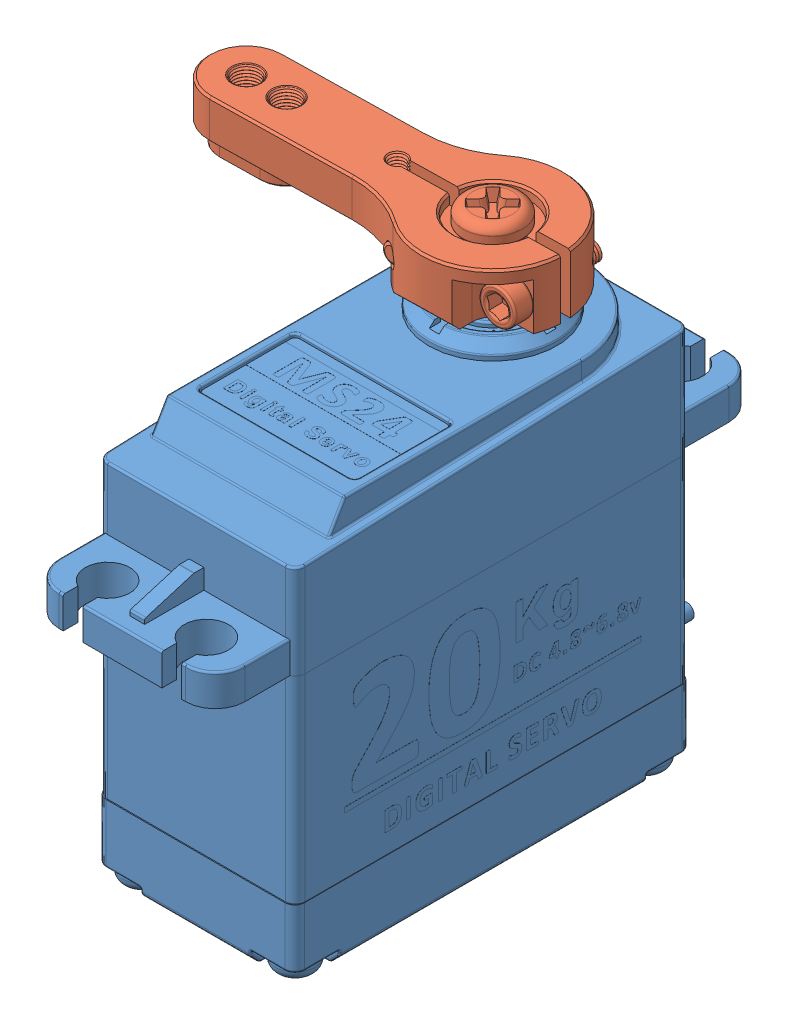
SolidWorks assembly servo, configuration Default. Lengths in mm.
Overall size (38.48 49.37 55.6).
2 component instances, 2 part files, 2 mates.
Components (placement in the parent):
- DS3218MG MS24 Digital Servo 270^servo-1: DS3218MG MS24 Digital Servo 270^servo [Default] at origin size (20.1 45.99 55.6) (virtual)
- Servo Arm^servo-1: Servo Arm^servo [Default] x (-0.018595 0 -0.999827) z (0.999827 0 -0.018595) size (14.5 6.95 35.53) (virtual)
Mates (geometry in assembly coordinates):
- Concentric1: concentric anti-aligned: cylinder of Servo Arm^DS3240 Digital Servo-1 through (0 18.4 0) axis (0 -1 0) radius 2.5; cylinder of DS3218MG MS24 Digital Servo 270-1 through (0 13.5 0) axis (0 1 0) radius 3.8
- Coincident1: coincident anti-aligned: plane of Copy of DS3218MG MS24 Digital Servo 270^DS3240 Digital Servo-1 through (0 18.4 0) normal (0 1 0); plane of Servo Arm^DS3240 Digital Servo-1 through (0 18.4 0) normal (0 -1 0)
